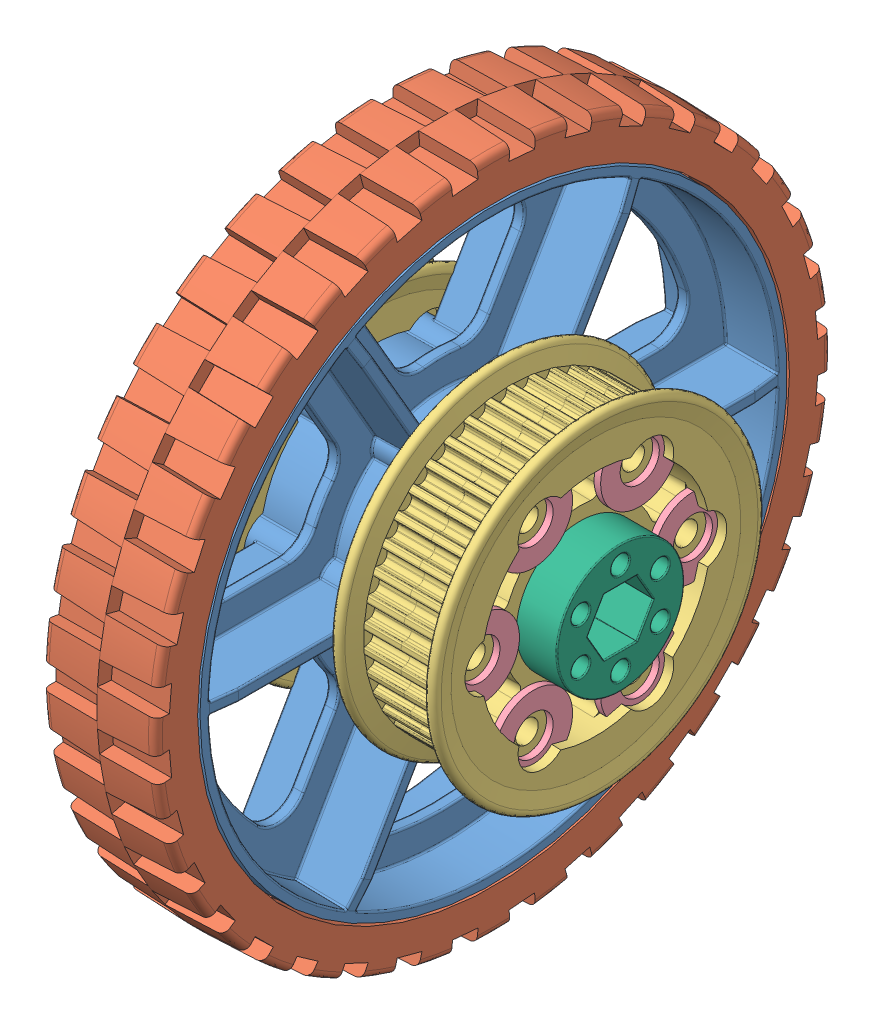
SolidWorks assembly 6 HiGrip with hub and double pulley, configuration Default. Lengths in mm.
Overall size (80.63 152.4 152.4).
21 component instances, 6 part files, 0 mates.
Components (placement in the parent):
- 6 HiGrip Wheel Assembly Rev II-1: 6 HiGrip Wheel Assembly Rev II [Default] at (83.7987 67.439 110.9939) size (34.93 152.4 152.4)
  - 6 wheel Rev 4-1: 6 wheel Rev 4 [Default] at (-52.6446 9.4231 21.378) size (34.93 132.08 132.08)
  - 6 wheel tread II-1: 6 wheel tread II [Default] at (-65.3446 9.4231 21.378) x (0 0 -1) z (1 0 0) size (152.4 152.4 25.58)
- HalfPulley_42t5mm-1: HalfPulley_42t5mm [Default] at (47.6006 76.862 132.3719) x (1 0 0) z (0 -0.5 0.866025) size (13 74.23 74.23)
- HalfPulley_42t5mm-2: HalfPulley_42t5mm [Default] at (64.263 76.862 132.3719) x (-1 0 0) z (0 -0.499927 0.866067) size (13 74.23 74.23)
- Washer_5-16-1: Washer_5-16 [Default] at (63.247 76.8605 108.5602) x (0 -0.812665 -0.582732) z (1 0 0) size (17.53 17.53 1.47)
- Washer_5-16-2: Washer_5-16 [Default] at (63.247 97.4833 120.4656) x (0 0.998209 0.059825) z (1 0 0) size (17.53 17.53 1.47)
- Washer_5-16-3: Washer_5-16 [Default] at (63.247 56.2398 144.2799) x (0 -0.026074 -0.99966) z (1 0 0) size (17.53 17.53 1.47)
- Washer_5-16-4: Washer_5-16 [Default] at (63.247 76.8625 156.1852) x (0 -0.766208 -0.642593) z (1 0 0) size (17.53 17.53 1.47)
- Washer_5-16-5: Washer_5-16 [Default] at (63.247 97.4843 144.2781) x (0 -0.833184 -0.552996) z (1 0 0) size (17.53 17.53 1.47)
- Washer_5-16-6: Washer_5-16 [Default] at (63.247 56.2388 120.4674) x (0 -0.998572 0.053424) z (1 0 0) size (17.53 17.53 1.47)
- HalfPulley_42t5mm-3: HalfPulley_42t5mm [Default] at (-1.9548 76.8628 132.3714) x (1 0 0) z (0 -1 -0.000063) size (13 74.23 74.23)
- HalfPulley_42t5mm-4: HalfPulley_42t5mm [Default] at (14.7076 76.8628 132.3714) x (-1 0 0) z (0 -1 0.000021) size (13 74.23 74.23)
- HexHub_500EX-1: HexHub_500EX [Default] at (-8.3048 76.862 132.3719) x (0 -0.866025 -0.5) z (0 -0.5 0.866025) size (55.37 25.4 51.33)
- Washer_5-16-7: Washer_5-16 [Default] at (-5.2568 97.4843 120.4656) x (0 0.577286 0.816542) z (-1 0 0) size (17.53 17.53 1.47)
- Washer_5-16-8: Washer_5-16 [Default] at (-5.2568 76.862 108.5594) x (0 0.877244 0.480045) z (-1 0 0) size (17.53 17.53 1.47)
- Washer_5-16-9: Washer_5-16 [Default] at (-5.2568 56.2398 120.4656) x (0 -0.894136 -0.447796) z (-1 0 0) size (17.53 17.53 1.47)
- Washer_5-16-10: Washer_5-16 [Default] at (-5.2568 97.4843 144.2781) x (0 -0.559623 -0.828747) z (-1 0 0) size (17.53 17.53 1.47)
- Washer_5-16-11: Washer_5-16 [Default] at (-5.2568 56.2398 144.2781) x (0 -0.82184 -0.569719) z (-1 0 0) size (17.53 17.53 1.47)
- Washer_5-16-12: Washer_5-16 [Default] at (-5.2568 76.862 156.1844) x (0 -0.981812 0.189856) z (-1 0 0) size (17.53 17.53 1.47)
- Spacer_Hex_0.57x0.5-1: Spacer_Hex_0.57x0.5 [Default] at (57.8495 76.862 132.3719) x (0 -0.866025 -0.5) z (0 -0.5 0.866025) size (28.55 14.48 28.55)
